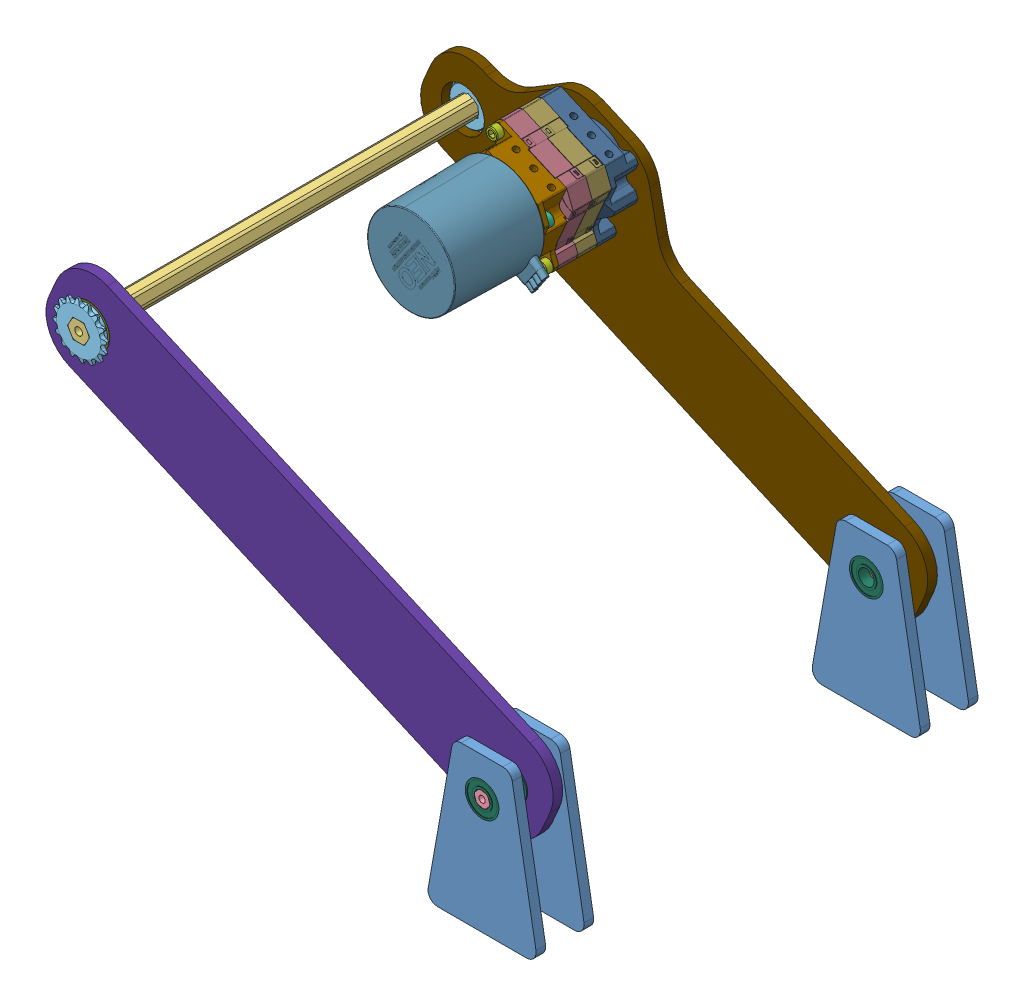
SolidWorks assembly intakeassembly - Copy, configuration Default. Lengths in mm.
Overall size (369.11 277.99 292.1).
35 component instances, 18 part files, 50 mates.
Components (placement in the parent):
- layout_sketch (2)-2: layout_sketch (2) [Default] at (16.0396 36.7133 123.2199) size (71.49 101.6 6.35)
- layout_sketch (2)-3: layout_sketch (2) [Default] at (16.0396 36.7133 -99.0301) size (71.49 101.6 6.35)
- 1_2thunderhex_1.5in-1: 1_2thunderhex_1.5in [Default] at (53.0044 112.9133 -556.2301) x (-0.618535 -0.785757 0) z (0 0 1) size (13.74 12.75 31.75)
- 1_2thunderhex_10.5in-1: 1_2thunderhex_10.5in [Default] at (-226.4054 234.7049 -308.5801) x (-0.456167 0.889894 0) z (0 0 1) size (13.74 12.75 266.7)
- 3_8thunderhex_1.5in-1: 3_8thunderhex_1.5in [Default] at (53.0044 112.9133 -295.8801) x (0.332678 -0.943041 0) z (0 0 1) size (10.24 9.53 38.1)
- 16T_#25_500_hex_hubbed_sprocket_217-2642-1: 16T_#25_500_hex_hubbed_sprocket_217-2642 [Default] at (-226.4054 234.7049 145.8259) x (-0.877701 0.479208 0) z (0 0 1) size (35.21 35.21 9.18)
- MAXPlanetary 2-Stage-1: MAXPlanetary 2-Stage [Default] at (-138.895 251.9764 -51.4051) x (-0.916699 0.399579 0) z (0 0 -1) size (89.61 89.51 122.08)
  - MAXPlanetary 2-Stage.STEP-1: MAXPlanetary 2-Stage.STEP [Default] at origin size (89.61 89.51 122.08)
    - REV-25-2109_2-Stage (No Shaft, For NEO).STEP-1: REV-25-2109_2-Stage (No Shaft, For NEO).STEP [Default] at origin size (65.15 54.03 73.34)
      - REV-25-2107_2-Stage.STEP-1: REV-25-2107_2-Stage.STEP [Default] at (0 0 6.35) x (-1 0 0) z (0 0 -1) size (65.15 54.03 73.34)
        - #10 Socket Head Cap Screws_0.500in Long.STEP-1: #10 Socket Head Cap Screws_0.500in Long.STEP [Default] at (21.1355 14.0872 12.7) x (0.923728 0.383049 0) z (0.383049 -0.923728 0) size (7.94 17.53 7.94)
        - #10 Socket Head Cap Screws_0.500in Long.STEP-2: #10 Socket Head Cap Screws_0.500in Long.STEP [Default] at (-21.1355 -14.0872 12.7) x (0.923728 0.383049 0) z (0.383049 -0.923728 0) size (7.94 17.53 7.94)
        - #10 Socket Head Cap Screws_1.500in Long.STEP-1: #10 Socket Head Cap Screws_1.500in Long.STEP [Default] at (-26.9919 21.4312 0) x (0.777574 0.628792 0) z (-0.628792 0.777574 0) size (7.94 42.93 7.94)
        - #10 Socket Head Cap Screws_1.500in Long.STEP-2: #10 Socket Head Cap Screws_1.500in Long.STEP [Default] at (26.9919 -21.4312 0) x (0.777574 0.628792 0) z (-0.628792 0.777574 0) size (7.94 42.93 7.94)
        - #10-32 Button Head Cap Screws_0.500in Long.STEP-1: #10-32 Button Head Cap Screws_0.500in Long.STEP [Default] at (0 0 -35.2425) x (0.655967 -0.754789 0) z (-0.754789 -0.655967 0) size (9.17 15.27 9.17)
      - REV-21-2106.STEP-1: REV-21-2106.STEP [Default] at origin size (61.91 50.8 19.05)
      - REV-21-2104.STEP-1: REV-21-2104.STEP [Default] at (0 0 44.45) x (0 0 1) z (-1 0 0) size (23.2 50.8 61.92)
      - REV-21-2108.STEP-1: REV-21-2108.STEP [Default] at (0 0 7.0985) x (-0.554615 -0.832107 0) z (0 0 -1) size (25.4 25.4 14.94)
    - REV-21-2101.STEP-1: REV-21-2101.STEP [Default] at (0 0 28.575) size (61.91 50.8 16.85)
    - REV-21-2102.STEP-1: REV-21-2102.STEP [Default] at (0 0 15.875) size (61.91 50.8 16.85)
    - REV-21-1650.STEP-1: REV-21-1650.STEP [Default] at (0 0 -9.525) x (0.554615 0.832107 0) z (0 0 1) size (64.41 64.76 93.26)
- thunderhex_375_flanged_217-5829-1: thunderhex_375_flanged_217-5829 [Default] at (53.0044 112.9133 154.2079) x (0 0 1) z (-0.756545 -0.653942 0) size (7.11 24.61 24.61)
- thunderhex_375_flanged_217-5829-2: thunderhex_375_flanged_217-5829 [Default] at (53.0044 112.9133 -123.6681) x (0 0 -1) z (-0.718679 0.695342 0) size (7.11 24.61 24.61)
- thunderhex_flanged_217-4006-2: thunderhex_flanged_217-4006 [Default] at (-226.4054 234.7049 138.3012) x (-1 0 0) z (0 0 -1) size (31.12 31.12 7.94)
- layout_sketch (2)-4: layout_sketch (2) [Default] at (16.0396 36.7133 154.9699) size (71.49 101.6 6.35)
- layout_sketch (2)-5: layout_sketch (2) [Default] at (16.0396 36.7133 -130.7801) size (71.49 101.6 6.35)
- thunderhex_375_flanged_217-5829-3: thunderhex_375_flanged_217-5829 [Default] at (53.0044 112.9133 130.3319) x (0 0 -1) z (-0.959715 -0.280976 0) size (7.11 24.61 24.61)
- thunderhex_375_flanged_217-5829-5: thunderhex_375_flanged_217-5829 [Default] at (53.0044 112.9133 -99.7921) x (0 0 1) z (-0.999866 -0.016349 0) size (7.11 24.61 24.61)
- thunderhex_375_flanged_217-5829-6: thunderhex_375_flanged_217-5829 [Default] at (53.0044 112.9133 135.9199) x (0 0 1) z (-0.999379 0.03525 0) size (7.11 24.61 24.61)
- thunderhex_375_flanged_217-5829-7: thunderhex_375_flanged_217-5829 [Default] at (53.0044 112.9133 -105.3801) x (0 0 -1) z (-0.879404 0.476076 0) size (7.11 24.61 24.61)
- layout_sketch (1)-1: layout_sketch (1) [Default] at (56.4421 28.2905 142.2699) x (-0.916699 0.399579 0) z (0 0 -1) size (355.6 63.5 6.35)
- layout_sketch-1: layout_sketch [Default] at (56.4421 28.2905 -105.3801) x (-0.916699 0.399579 0) z (0 0 -1) size (355.6 107.95 6.35)
- 16T_#25_500_hex_hubbed_sprocket_217-2642-2: 16T_#25_500_hex_hubbed_sprocket_217-2642 [Default] at (-226.4054 234.7049 -115.2861) x (-1 0 0) z (0 0 -1) size (35.21 35.21 9.18)
- 16T_#25_500_hex_hubbed_sprocket_217-2642-3: 16T_#25_500_hex_hubbed_sprocket_217-2642 [Default] at (-138.895 251.9764 -115.2861) x (-0.723016 -0.690831 0) z (0 0 -1) size (35.21 35.21 9.18)
- 1_2thunderhex_1.5in-2: 1_2thunderhex_1.5in [Default] at (-138.895 251.9764 -543.5301) x (0.99729 -0.073573 0) z (0 0 1) size (13.74 12.75 31.75)
Mates (geometry in assembly coordinates):
- Parallel1: parallel aligned: line of layout_sketch (2)-2 through (23.6073 36.7133 129.5699) axis (1 0 0); line of layout_sketch (2)-3 through (23.6073 36.7133 -92.6801) axis (1 0 0)
- Parallel3: parallel aligned: plane of layout_sketch (2)-2 through (39.2827 138.3133 129.5699) normal (0 1 0); plane of layout_sketch (2)-3 through (39.2827 138.3133 -92.6801) normal (0 1 0)
- Distance1: distance = 222.25 mm aligned: plane of layout_sketch (2)-3 through (82.4016 43.0633 -92.6801) normal (0 0 1); plane of layout_sketch (2)-2 through (82.4016 43.0633 129.5699) normal (0 0 1)
- Coincident3: coincident aligned: plane of layout_sketch (2)-2 through (39.2827 138.3133 129.5699) normal (0 1 0); plane of layout_sketch (2)-3 through (39.2827 138.3133 -92.6801) normal (0 1 0)
- Coincident4: coincident aligned: plane of layout_sketch (2)-2 through (72.9797 133.0659 129.5699) normal (0.984808 0.173648 0); plane of layout_sketch (2)-3 through (72.9797 133.0659 -92.6801) normal (0.984808 0.173648 0)
- Parallel6: parallel aligned: plane of layout_sketch (2)-2 through (39.2827 138.3133 129.5699) normal (0 1 0); plane of layout_sketch (2)-4 through (39.2827 138.3133 161.3199) normal (0 1 0)
- Parallel7: parallel aligned: plane of layout_sketch (2)-2 through (72.9797 133.0659 129.5699) normal (0.984808 0.173648 0); plane of layout_sketch (2)-4 through (72.9797 133.0659 161.3199) normal (0.984808 0.173648 0)
- Coincident14: coincident aligned: plane of layout_sketch (2)-2 through (72.9797 133.0659 129.5699) normal (0.984808 0.173648 0); plane of layout_sketch (2)-4 through (72.9797 133.0659 161.3199) normal (0.984808 0.173648 0)
- Coincident15: coincident aligned: plane of layout_sketch (2)-2 through (39.2827 138.3133 129.5699) normal (0 1 0); plane of layout_sketch (2)-4 through (39.2827 138.3133 161.3199) normal (0 1 0)
- Coincident16: coincident aligned: plane of layout_sketch (2)-3 through (39.2827 138.3133 -92.6801) normal (0 1 0); plane of layout_sketch (2)-5 through (39.2827 138.3133 -124.4301) normal (0 1 0)
- Coincident17: coincident aligned: plane of layout_sketch (2)-3 through (72.9797 133.0659 -92.6801) normal (0.984808 0.173648 0); plane of layout_sketch (2)-5 through (72.9797 133.0659 -124.4301) normal (0.984808 0.173648 0)
- Coincident20: coincident aligned: plane of layout_sketch (2)-3 through (82.4016 43.0633 -92.6801) normal (0 0 1); plane of thunderhex_375_flanged_217-5829-5 through (52.8425 122.8179 -92.6801) normal (0 0 1)
- Concentric9: concentric aligned: cylinder of layout_sketch (2)-3 through (53.0044 112.9133 -92.6801) axis (0 0 -1) radius 11.1125; cylinder of thunderhex_375_flanged_217-5829-5 through (53.0044 112.9133 -99.7921) axis (0 0 -1) radius 5.125
- Coincident23: coincident aligned: plane of thunderhex_375_flanged_217-5829-2 through (46.1164 105.794 -130.7801) normal (0 0 -1); plane of layout_sketch (2)-5 through (82.4016 43.0633 -130.7801) normal (0 0 -1)
- Concentric10: concentric anti-aligned: cylinder of thunderhex_375_flanged_217-5829-2 through (53.0044 112.9133 -123.6681) axis (0 0 1) radius 5.125; cylinder of layout_sketch (2)-5 through (53.0044 112.9133 -124.4301) axis (0 0 -1) radius 11.1125
- Coincident27: coincident aligned: plane of layout_sketch (2)-2 through (82.4016 43.0633 123.2199) normal (0 0 -1); plane of thunderhex_375_flanged_217-5829-3 through (55.7878 103.4063 123.2199) normal (0 0 -1)
- Concentric13: concentric anti-aligned: cylinder of layout_sketch (2)-2 through (53.0044 112.9133 129.5699) axis (0 0 -1) radius 11.1125; cylinder of thunderhex_375_flanged_217-5829-3 through (53.0044 112.9133 130.3319) axis (0 0 1) radius 5.125
- Coincident31: coincident aligned: plane of thunderhex_375_flanged_217-5829-1 through (46.5265 120.4076 161.3199) normal (0 0 1); plane of layout_sketch (2)-4 through (82.4016 43.0633 161.3199) normal (0 0 1)
- Concentric15: concentric anti-aligned: cylinder of thunderhex_375_flanged_217-5829-1 through (53.0044 112.9133 154.2079) axis (0 0 -1) radius 5.125; circle of layout_sketch (2)-4
- Distance2: distance = 31.75 mm aligned: plane of layout_sketch (2)-2 through (82.4016 43.0633 129.5699) normal (0 0 1); plane of layout_sketch (2)-4 through (82.4016 43.0633 161.3199) normal (0 0 1)
- Distance3: distance = 31.75 mm aligned: plane of layout_sketch (2)-5 through (82.4016 43.0633 -124.4301) normal (0 0 1); plane of layout_sketch (2)-3 through (82.4016 43.0633 -92.6801) normal (0 0 1)
- Coincident34: coincident aligned: plane of 3_8thunderhex_1.5in-1 through (53.0044 112.9133 161.3199) normal (0 0 1); plane of layout_sketch (2)-4 through (82.4016 43.0633 161.3199) normal (0 0 1)
- Concentric16: concentric anti-aligned: cylinder of 3_8thunderhex_1.5in-1 through (53.0044 112.9133 -753.0801) axis (0 0 1) radius 2.1; cylinder of thunderhex_375_flanged_217-5829-1 through (53.0044 112.9133 154.2079) axis (0 0 -1) radius 5.125
- Coincident36: coincident aligned: plane of 1_2thunderhex_1.5in-1 through (88.5441 168.3684 -130.7801) normal (0 0 -1); plane of layout_sketch (2)-5 through (82.4016 43.0633 -130.7801) normal (0 0 -1)
- Concentric17: concentric aligned: cylinder of 1_2thunderhex_1.5in-1 through (53.0044 112.9133 -1013.4301) axis (0 0 1) radius 2.55; cylinder of thunderhex_375_flanged_217-5829-2 through (53.0044 112.9133 -123.6681) axis (0 0 1) radius 5.125
- Concentric18: concentric aligned: cylinder of 1_2thunderhex_1.5in-1 through (53.0044 112.9133 -1013.4301) axis (0 0 1) radius 2.55; cylinder of thunderhex_375_flanged_217-5829-7 through (53.0044 112.9133 -105.3801) axis (0 0 1) radius 5.125
- Concentric19: concentric anti-aligned: cylinder of 3_8thunderhex_1.5in-1 through (53.0044 112.9133 -753.0801) axis (0 0 1) radius 2.1; cylinder of thunderhex_375_flanged_217-5829-6 through (53.0044 112.9133 135.9199) axis (0 0 -1) radius 5.125
- Distance6: distance = 12.7 mm aligned: plane of thunderhex_375_flanged_217-5829-7 through (47.1457 102.0911 -105.3801) normal (0 0 1); plane of layout_sketch (2)-3 through (82.4016 43.0633 -92.6801) normal (0 0 1)
- Distance7: distance = 12.7 mm aligned: plane of layout_sketch (2)-2 through (82.4016 43.0633 123.2199) normal (0 0 -1); plane of thunderhex_375_flanged_217-5829-6 through (53.4382 125.2119 135.9199) normal (0 0 -1)
- Concentric20: concentric aligned: cylinder of thunderhex_375_flanged_217-5829-7 through (53.0044 112.9133 -105.3801) axis (0 0 1) radius 11.1125; cylinder of layout_sketch-1 through (53.0044 112.9133 -111.7301) axis (0 0 1) radius 11.1125
- Concentric21: concentric aligned: cylinder of 3_8thunderhex_1.5in-1 through (53.0044 112.9133 -753.0801) axis (0 0 1) radius 2.1; cylinder of layout_sketch (1)-1 through (53.0044 112.9133 135.9199) axis (0 0 1) radius 11.1125
- Parallel9: parallel aligned: plane of layout_sketch (1)-1 through (65.6911 142.0185 135.9199) normal (0.399579 0.916699 0); plane of layout_sketch-1 through (65.6911 142.0185 -111.7301) normal (0.399579 0.916699 0)
- Coincident47: coincident aligned: plane of thunderhex_375_flanged_217-5829-6 through (53.4382 125.2119 135.9199) normal (0 0 -1); plane of layout_sketch (1)-1 through (-228.9427 228.8839 135.9199) normal (0 0 -1)
- Coincident48: coincident aligned: plane of thunderhex_375_flanged_217-5829-7 through (47.1457 102.0911 -105.3801) normal (0 0 1); plane of layout_sketch-1 through (-228.9427 228.8839 -105.3801) normal (0 0 1)
- Concentric23: concentric aligned: cylinder of 1_2thunderhex_10.5in-1 through (-226.4054 234.7049 -765.7801) axis (0 0 1) radius 2.55; cylinder of layout_sketch (1)-1 through (-226.4054 234.7049 135.9199) axis (0 0 1) radius 14.2875
- Distance8: distance = 6.35 mm aligned: plane of 1_2thunderhex_10.5in-1 through (-226.4054 234.7049 148.6199) normal (0 0 1); plane of layout_sketch (1)-1 through (-228.9427 228.8839 142.2699) normal (0 0 1)
- Coincident51: coincident aligned: plane of thunderhex_flanged_217-4006-2 through (-226.4054 246.9924 142.2699) normal (0 0 1); plane of layout_sketch (1)-1 through (-228.9427 228.8839 142.2699) normal (0 0 1)
- Concentric24: concentric anti-aligned: cylinder of thunderhex_flanged_217-4006-2 through (-226.4054 234.7049 85.0522) axis (0 0 -1) radius 6.875; cylinder of layout_sketch (1)-1 through (-226.4054 234.7049 135.9199) axis (0 0 1) radius 14.2875
- Concentric26: concentric anti-aligned: cylinder of 16T_#25_500_hex_hubbed_sprocket_217-2642-1 through (-226.4054 234.7049 139.4442) axis (0 0 1) radius 12.7; cylinder of thunderhex_flanged_217-4006-2 through (-226.4054 234.7049 85.0522) axis (0 0 -1) radius 14.2875
- Concentric27: concentric aligned: circle of 16T_#25_500_hex_hubbed_sprocket_217-2642-1; circle of thunderhex_flanged_217-4006-2
- Coincident53: coincident aligned: plane of 1_2thunderhex_10.5in-1 through (-226.4054 234.7049 148.6199) normal (0 0 1); plane of 16T_#25_500_hex_hubbed_sprocket_217-2642-1 through (-226.4054 234.7049 148.6199) normal (0 0 1)
- Concentric28: concentric anti-aligned: cylinder of 1_2thunderhex_10.5in-1 through (-226.4054 234.7049 -765.7801) axis (0 0 1) radius 2.55; cylinder of 16T_#25_500_hex_hubbed_sprocket_217-2642-2 through (-226.4054 234.7049 -108.9043) axis (0 0 -1) radius 12.7
- Coincident55: coincident aligned: plane of 1_2thunderhex_10.5in-1 through (-190.8271 179.2746 -118.0801) normal (0 0 -1); plane of 16T_#25_500_hex_hubbed_sprocket_217-2642-2 through (-226.4054 234.7049 -118.0801) normal (0 0 -1)
- Coincident56: coincident anti-aligned: plane of MAXPlanetary 2-Stage-1/MAXPlanetary 2-Stage.STEP-1/REV-25-2109_2-Stage (No Shaft, For NEO).STEP-1/REV-21-2104.STEP-1 through (-138.895 251.9764 -105.3801) normal (0 0 -1); plane of layout_sketch-1 through (-228.9427 228.8839 -105.3801) normal (0 0 1)
- Parallel10: parallel aligned: plane of MAXPlanetary 2-Stage-1/MAXPlanetary 2-Stage.STEP-1/REV-25-2109_2-Stage (No Shaft, For NEO).STEP-1/REV-21-2104.STEP-1 through (-152.0299 285.4098 -86.3301) normal (0.399579 0.916699 0); plane of layout_sketch-1 through (65.6911 142.0185 -111.7301) normal (0.399579 0.916699 0)
- Concentric29: concentric aligned: cylinder of MAXPlanetary 2-Stage-1/MAXPlanetary 2-Stage.STEP-1/REV-25-2109_2-Stage (No Shaft, For NEO).STEP-1/REV-25-2107_2-Stage.STEP-1/#10-32 Button Head Cap Screws_0.500in Long.STEP-1 through (-138.895 251.9764 -92.3753) axis (0 0 1) radius 2.413; cylinder of layout_sketch-1 through (-138.895 251.9764 -111.7301) axis (0 0 1) radius 12.7
- Coincident58: coincident aligned: plane of 1_2thunderhex_10.5in-1 through (-190.8271 179.2746 -118.0801) normal (0 0 -1); plane of 1_2thunderhex_1.5in-2 through (-204.7432 250.4414 -118.0801) normal (0 0 -1)
- Concentric30: concentric aligned: cylinder of MAXPlanetary 2-Stage-1/MAXPlanetary 2-Stage.STEP-1/REV-25-2109_2-Stage (No Shaft, For NEO).STEP-1/REV-25-2107_2-Stage.STEP-1/#10-32 Button Head Cap Screws_0.500in Long.STEP-1 through (-138.895 251.9764 -92.3753) axis (0 0 1) radius 2.413; cylinder of 1_2thunderhex_1.5in-2 through (-138.895 251.9764 -1000.7301) axis (0 0 1) radius 2.55
- Coincident59: coincident aligned: plane of 16T_#25_500_hex_hubbed_sprocket_217-2642-2 through (-226.4054 234.7049 -118.0801) normal (0 0 -1); plane of 16T_#25_500_hex_hubbed_sprocket_217-2642-3 through (-138.895 251.9764 -118.0801) normal (0 0 -1)
- Concentric31: concentric anti-aligned: cylinder of 16T_#25_500_hex_hubbed_sprocket_217-2642-3 through (-138.895 251.9764 -108.9043) axis (0 0 -1) radius 12.7; cylinder of 1_2thunderhex_1.5in-2 through (-138.895 251.9764 -1000.7301) axis (0 0 1) radius 2.55
